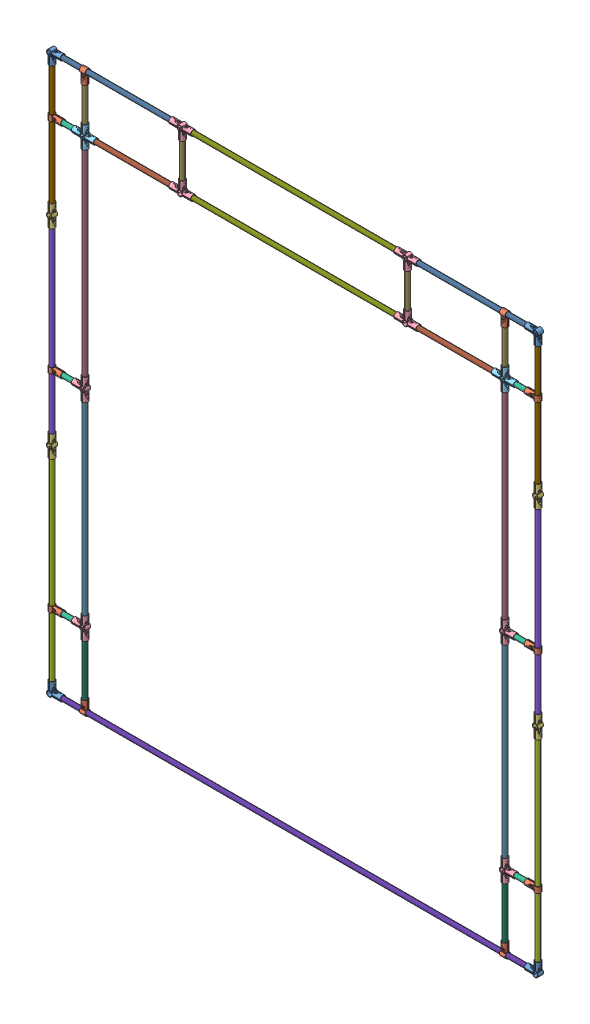
SolidWorks assembly End_Panel_Assembly, configuration Default. Lengths in mm.
Overall size (2924.59 3334.67 35.62).
57 component instances, 17 part files, 65 mates.
Components (placement in the parent):
- 28-25-3: 28-25 [2534T24] x (0 1 0) z (0 0 1) size (81.85 81.28 33.46)
- 28-20-9: 28-20 [2534T21] at (196 0 0) x (1 0 0) z (0 0 -1) size (33.53 82.55 34.1)
- 28-20-10: 28-20 [2534T21] at (0 436 0) x (0 -1 0) z (0 0 -1) size (33.53 82.55 34.1)
- 28-22-2: 28-22 [2534T25] at (0 1275 0) x (0 -1 0) z (0 0 1) size (130.05 34.67 33.46)
- 28-20-8: 28-20 [2534T21] at (0 1665 0) x (0 -1 0) z (0 0 -1) size (33.53 82.55 34.1)
- 24-25-4: 24-25 [2534T26] at (196 1665 0) x (0 1 0) z (0 0 -1) size (130.05 82.36 33.46)
- 28-22-3: 28-22 [2534T25] at (0 2461 0) x (0 -1 0) z (0 0 1) size (130.05 34.67 33.46)
- 28-24-3: 28-24 [2534T27] at (196 2965 0) size (130.05 130.05 33.46)
- 28-20-7: 28-20 [2534T21] at (0 2965 0) x (0 -1 0) z (0 0 -1) size (33.53 82.55 34.1)
- 24-25-24: 24-25 [2534T26] at (775 2965 0) x (1 0 0) z (0 0 -1) size (130.05 82.36 33.46)
- 28-25-5: 28-25 [2534T24] at (0 3300 0) size (81.85 81.28 33.46)
- 28-20-6: 28-20 [2534T21] at (196 3300 0) size (33.53 82.55 34.1)
- 24-25-25: 24-25 [2534T26] at (775 3300 0) size (130.05 82.36 33.46)
- 28-02-2: 28-02 [Default] at (43.381 436 0) size (110 25.4 25.4)
- 28-02-3: 28-02 [Default] at (43.381 1665 0) x (1 0 0) z (0 -0.125641 0.992076) size (110 25.4 25.4)
- 28-02-4: 28-02 [Default] at (43.381 2965 0) size (110 25.4 25.4)
- 28-03-1: 28-03 [Default] at (0 42.246 0) x (0 1 0) z (0 0 1) size (1190 25.4 25.4)
- 28-04-2: 28-04 [Default] at (0 2418 0) x (0 -1 0) z (-0.79674 0 -0.604323) size (1100 25.4 25.4)
- 28-05-1: 28-05 [Default] at (0 3255.754 0) x (0 -1 0) z (0.421273 0 0.906934) size (750 25.4 25.4)
- 28-06-1: 28-06 [Default] at (42.246 3300 0) size (690 25.4 25.4)
- 28-07-1: 28-07 [Default] at (240.5 2965 0) size (490 25.4 25.4)
- 28-08-1: 28-08 [Default] at (196 3254.619 0) x (0 -1 0) z (-0.507156 0 0.861854) size (245 25.4 25.4)
- 28-08-2: 28-08 [Default] at (775 3255 0) x (0 -1 0) z (0.98977 0 -0.14267) size (245 25.4 25.4)
- 28-09-1: 28-09 [Default] at (196 2920 0) x (0 -1 0) z (-0.937477 0 0.348048) size (1210 25.4 25.4)
- 28-10-1: 28-10 [Default] at (196 1620.5 0) x (0 -1 0) z (0.792816 0 0.609461) size (1140 25.4 25.4)
- 28-12-1: 28-12 [Default] at (196 45.881 0) x (0 1 0) z (0.833818 0 0.552039) size (345 25.4 25.4)
- 28-16-1: 28-16 [Default] at (819.25 3300 0) size (1250 25.4 25.4)
- 28-16-2: 28-16 [Default] at (819.5 2965 0) size (1250 25.4 25.4)
- 28-12-9: 28-12 [Default] at (2693 45.881 0) x (0 1 0) z (0.833818 0 -0.552039) size (345 25.4 25.4)
- 28-03-6: 28-03 [Default] at (2889 42.246 0) x (0 1 0) z (0 0 -1) size (1190 25.4 25.4)
- 28-25-15: 28-25 [2534T24] at (2889 0 0) x (0 1 0) z (0 0 -1) size (81.85 81.28 33.46)
- 28-20-27: 28-20 [2534T21] at (2693 0 0) x (1 0 0) z (0 0 -1) size (33.53 82.55 34.1)
- 28-02-17: 28-02 [Default] at (2845.619 436 0) x (-1 0 0) z (0 0 -1) size (110 25.4 25.4)
- 28-20-28: 28-20 [2534T21] at (2889 436 0) x (0 1 0) z (0 0 -1) size (33.53 82.55 34.1)
- 28-10-6: 28-10 [Default] at (2693 1620.5 0) x (0 -1 0) z (0.792816 0 -0.609461) size (1140 25.4 25.4)
- 28-22-12: 28-22 [2534T25] at (2889 1275 0) x (0 -1 0) z (0 0 -1) size (130.05 34.67 33.46)
- 28-04-7: 28-04 [Default] at (2889 2418 0) x (0 -1 0) z (-0.79674 0 0.604323) size (1100 25.4 25.4)
- 24-25-26: 24-25 [2534T26] at (2693 1665 0) x (0 1 0) z (0 0 1) size (130.05 82.36 33.46)
- 28-02-18: 28-02 [Default] at (2845.619 1665 0) x (-1 0 0) z (0 0.125641 -0.992076) size (110 25.4 25.4)
- 28-20-29: 28-20 [2534T21] at (2889 1665 0) x (0 1 0) z (0 0 -1) size (33.53 82.55 34.1)
- 28-09-6: 28-09 [Default] at (2693 2920 0) x (0 -1 0) z (-0.937477 0 -0.348048) size (1210 25.4 25.4)
- 28-22-13: 28-22 [2534T25] at (2889 2461 0) x (0 -1 0) z (0 0 -1) size (130.05 34.67 33.46)
- 28-05-6: 28-05 [Default] at (2889 3255.754 0) x (0 -1 0) z (0.421273 0 -0.906934) size (750 25.4 25.4)
- 28-08-11: 28-08 [Default] at (2114 3255 0) x (0 -1 0) z (0.98977 0 0.14267) size (245 25.4 25.4)
- 24-25-27: 24-25 [2534T26] at (2114 2965 0) x (-1 0 0) z (0 0 1) size (130.05 82.36 33.46)
- 28-07-6: 28-07 [Default] at (2648.5 2965 0) x (-1 0 0) z (0 0 -1) size (490 25.4 25.4)
- 28-24-13: 28-24 [2534T27] at (2693 2965 0) x (-1 0 0) z (0 0 -1) size (130.05 130.05 33.46)
- 28-02-19: 28-02 [Default] at (2845.619 2965 0) x (-1 0 0) z (0 0 -1) size (110 25.4 25.4)
- 28-20-30: 28-20 [2534T21] at (2889 2965 0) x (0 1 0) z (0 0 -1) size (33.53 82.55 34.1)
- 28-08-12: 28-08 [Default] at (2693 3254.619 0) x (0 -1 0) z (-0.507156 0 -0.861854) size (245 25.4 25.4)
- 28-25-16: 28-25 [2534T24] at (2889 3300 0) x (-1 0 0) z (0 0 -1) size (81.85 81.28 33.46)
- 28-20-31: 28-20 [2534T21] at (2693 3300 0) size (33.53 82.55 34.1)
- 28-06-6: 28-06 [Default] at (2846.754 3300 0) x (-1 0 0) z (0 0 -1) size (690 25.4 25.4)
- 24-25-28: 24-25 [2534T26] at (2114 3300 0) x (-1 0 0) z (0 0 -1) size (130.05 82.36 33.46)
- 28-17-1: 28-17 [Default] at (44.5 0 0) size (2800 25.4 25.4)
- 24-25-23: 24-25 [2534T26] at (196 436 0) x (0 1 0) z (0 0 -1) size (130.05 82.36 33.46)
- 24-25-29: 24-25 [2534T26] at (2693 436 0) x (0 1 0) z (0 0 1) size (130.05 82.36 33.46)
Mates (geometry in assembly coordinates):
- Coincident26: coincident: unknown of 3way connector-3
- Parallel15: parallel aligned: plane of 3way connector-3 through (0 64.516 0) normal (0 1 0)
- Parallel16: parallel aligned: plane of 3way connector-3 through (64.516 0 0) normal (1 0 0)
- Concentric12: concentric aligned: cylinder of 3way connector-3 through (64.516 0 0) axis (-1 0 0) radius 13.97; cylinder of Tee connector-2 through (212.764 0 0) axis (-1 0 0) radius 13.97
- Distance10: distance = 196 mm: unknown of Tee connector-2
- Parallel17: parallel aligned: plane of Tee connector-2 through (196 65.786 0) normal (0 1 0)
- Concentric18: concentric aligned: cylinder of 3way connector-3 through (0 64.516 0) axis (0 -1 0) radius 13.97; cylinder of Tee connector-3 through (0 452.764 0) axis (0 -1 0) radius 13.97
- Concentric19: concentric anti-aligned: cylinder of Tee connector-3 through (0 452.764 0) axis (0 -1 0) radius 13.97; cylinder of Cross-2 through (0 1209.976 0) axis (0 1 0) radius 13.97
- Distance13: distance = 1275 mm: unknown of Cross-2
- Concentric24: concentric anti-aligned: cylinder of Cross-2 through (0 1340.024 0) axis (0 -1 0) radius 13.97; cylinder of Tee connector-4 through (0 1648.236 0) axis (0 1 0) radius 13.97
- Concentric26: concentric anti-aligned: cylinder of Tee connector-4 through (65.786 1665 0) axis (-1 0 0) radius 13.97; cylinder of 5way connector-4 through (130.976 1665 0) axis (1 0 0) radius 13.97
- Concentric28: concentric anti-aligned: cylinder of Tee connector-4 through (0 1681.764 0) axis (0 -1 0) radius 13.97; cylinder of Cross-3 through (0 2395.976 0) axis (0 1 0) radius 13.97
- Parallel21: parallel aligned: plane of Tee connector-4 through (25.146 1665 12.065) normal (0 0 1); plane of Cross-3 through (0 2461 16.73) normal (0 0 1)
- Distance18: distance = 1186 mm: point of Cross-3; point of Cross-2
- Parallel22: parallel aligned: plane of Cross-3 through (0 2461 16.73) normal (0 0 1); plane of 6way connector-3 through (196 2965 16.73) normal (0 0 1)
- Concentric29: concentric anti-aligned: cylinder of 5way connector-4 through (196 1730.024 0) axis (0 -1 0) radius 13.97; cylinder of 6way connector-3 through (196 2899.976 0) axis (0 1 0) radius 13.97
- Distance19: distance = 1300 mm: point of 6way connector-3; point of 5way connector-4
- Concentric30: concentric aligned: cylinder of Cross-3 through (0 2526.024 0) axis (0 -1 0) radius 13.97; cylinder of Tee connector-5 through (0 2981.764 0) axis (0 -1 0) radius 13.97
- Concentric31: concentric anti-aligned: cylinder of 6way connector-3 through (130.976 2965 0) axis (1 0 0) radius 13.97; cylinder of Tee connector-5 through (65.786 2965 0) axis (-1 0 0) radius 13.97
- Concentric35: concentric anti-aligned: cylinder of 6way connector-3 through (261.024 2965 0) axis (-1 0 0) radius 13.97; cylinder of 5way connector-5 through (709.976 2965 0) axis (1 0 0) radius 13.97
- Concentric36: concentric aligned: cylinder of 3way connector-5 through (64.516 3300 0) axis (-1 0 0) radius 13.97; cylinder of Tee connector-6 through (212.764 3300 0) axis (-1 0 0) radius 13.97
- Concentric37: concentric anti-aligned: cylinder of Tee connector-5 through (0 2981.764 0) axis (0 -1 0) radius 13.97; cylinder of 3way connector-5 through (0 3235.484 0) axis (0 1 0) radius 13.97
- Concentric38: concentric anti-aligned: cylinder of 6way connector-3 through (196 3030.024 0) axis (0 -1 0) radius 13.97; cylinder of Tee connector-6 through (196 3234.214 0) axis (0 1 0) radius 13.97
- Distance22: distance = 335 mm: point of 3way connector-5; point of Tee connector-5
- Concentric39: concentric anti-aligned: cylinder of Tee connector-6 through (212.764 3300 0) axis (-1 0 0) radius 13.97; cylinder of 5way connector-6 through (709.976 3300 0) axis (1 0 0) radius 13.97
- Concentric41: concentric anti-aligned: cylinder of 5way connector-5 through (775 3030.024 0) axis (0 -1 0) radius 13.97; cylinder of 5way connector-6 through (775 3234.976 0) axis (0 1 0) radius 13.97
- Concentric44: concentric aligned: cylinder of Tee connector-4 through (65.786 1665 0) axis (-1 0 0) radius 13.97; cylinder of P2-3 through (153.381 1665 0) axis (-1 0 0) radius 12.7
- Width3: width anti-aligned: plane of P2-3 through (153.381 1665 0) normal (1 0 0); plane of P2-3 through (43.381 1665 0) normal (-1 0 0); plane of 5way connector-4 through (130.976 1665 0) normal (-1 0 0); plane of Tee connector-4 through (65.786 1665 0) normal (1 0 0)
- Width4: width anti-aligned: plane of P2-4 through (153.381 2965 0) normal (1 0 0); plane of P2-4 through (43.381 2965 0) normal (-1 0 0); plane of 6way connector-3 through (130.976 2965 0) normal (-1 0 0); plane of Tee connector-5 through (65.786 2965 0) normal (1 0 0)
- Concentric45: concentric aligned: cylinder of Tee connector-5 through (65.786 2965 0) axis (-1 0 0) radius 13.97; cylinder of P2-4 through (153.381 2965 0) axis (-1 0 0) radius 12.7
- Concentric46: concentric anti-aligned: cylinder of Cross-2 through (0 1209.976 0) axis (0 1 0) radius 13.97; cylinder of P3-1 through (0 1232.246 0) axis (0 -1 0) radius 12.7
- Width5: width aligned: plane of P3-1 through (0 42.246 0) normal (0 -1 0); plane of P3-1 through (0 1232.246 0) normal (0 1 0); plane of Cross-2 through (0 1209.976 0) normal (0 -1 0); plane of 3way connector-3 through (0 64.516 0) normal (0 1 0)
- Concentric47: concentric anti-aligned: cylinder of Cross-2 through (0 1340.024 0) axis (0 -1 0) radius 13.97; cylinder of P4-2 through (0 1318 0) axis (0 1 0) radius 12.7
- Width6: width anti-aligned: plane of P4-2 through (0 2418 0) normal (0 1 0); plane of P4-2 through (0 1318 0) normal (0 -1 0); plane of Cross-3 through (0 2395.976 0) normal (0 -1 0); plane of Cross-2 through (0 1340.024 0) normal (0 1 0)
- Concentric48: concentric anti-aligned: cylinder of Cross-3 through (0 2526.024 0) axis (0 -1 0) radius 13.97; cylinder of P5-1 through (0 2505.754 0) axis (0 1 0) radius 12.7
- Width7: width anti-aligned: plane of P5-1 through (0 3255.754 0) normal (0 1 0); plane of P5-1 through (0 2505.754 0) normal (0 -1 0); plane of 3way connector-5 through (0 3235.484 0) normal (0 -1 0); plane of Cross-3 through (0 2526.024 0) normal (0 1 0)
- Width8: width anti-aligned: plane of P6-1 through (42.246 3300 0) normal (-1 0 0); plane of P6-1 through (732.246 3300 0) normal (1 0 0); plane of 3way connector-5 through (64.516 3300 0) normal (1 0 0); plane of 5way connector-6 through (709.976 3300 0) normal (-1 0 0)
- Concentric49: concentric anti-aligned: cylinder of 5way connector-6 through (709.976 3300 0) axis (1 0 0) radius 13.97; cylinder of P6-1 through (732.246 3300 0) axis (-1 0 0) radius 12.7
- Width9: width anti-aligned: plane of P7-1 through (240.5 2965 0) normal (-1 0 0); plane of P7-1 through (730.5 2965 0) normal (1 0 0); plane of 6way connector-3 through (261.024 2965 0) normal (1 0 0); plane of 5way connector-5 through (709.976 2965 0) normal (-1 0 0)
- Concentric50: concentric anti-aligned: cylinder of 5way connector-5 through (709.976 2965 0) axis (1 0 0) radius 13.97; cylinder of P7-1 through (730.5 2965 0) axis (-1 0 0) radius 12.7
- Concentric51: concentric anti-aligned: cylinder of 6way connector-3 through (196 3030.024 0) axis (0 -1 0) radius 13.97; cylinder of P8-1 through (196 3009.619 0) axis (0 1 0) radius 12.7
- Concentric52: concentric anti-aligned: cylinder of 5way connector-5 through (775 3030.024 0) axis (0 -1 0) radius 13.97; cylinder of P8-2 through (775 3010 0) axis (0 1 0) radius 12.7
- Width10: width aligned: plane of P8-1 through (196 3254.619 0) normal (0 1 0); plane of P8-1 through (196 3009.619 0) normal (0 -1 0); plane of 6way connector-3 through (196 3030.024 0) normal (0 1 0); plane of Tee connector-6 through (196 3234.214 0) normal (0 -1 0)
- Width11: width anti-aligned: plane of P8-2 through (775 3255 0) normal (0 1 0); plane of P8-2 through (775 3010 0) normal (0 -1 0); plane of 5way connector-6 through (775 3234.976 0) normal (0 -1 0); plane of 5way connector-5 through (775 3030.024 0) normal (0 1 0)
- Concentric53: concentric anti-aligned: cylinder of 5way connector-4 through (196 1730.024 0) axis (0 -1 0) radius 13.97; cylinder of P9-1 through (196 1710 0) axis (0 1 0) radius 12.7
- Width12: width anti-aligned: plane of P9-1 through (196 1710 0) normal (0 -1 0); plane of P9-1 through (196 2920 0) normal (0 1 0); plane of 5way connector-4 through (196 1730.024 0) normal (0 1 0); plane of 6way connector-3 through (196 2899.976 0) normal (0 -1 0)
- Width20: width anti-aligned: plane of P16-1 through (2069.25 3300 0) normal (1 0 0); plane of P16-1 through (819.25 3300 0) normal (-1 0 0); plane of 5way connector-10 through (2048.976 3250 0) normal (-1 0 0); plane of 5way connector-6 through (840.024 3300 0) normal (1 0 0)
- Width21: width anti-aligned: plane of P16-2 through (2069.5 2965 0) normal (1 0 0); plane of P16-2 through (819.5 2965 0) normal (-1 0 0); plane of 5way connector-9 through (2048.976 2915 0) normal (-1 0 0); plane of 5way connector-5 through (840.024 2965 0) normal (1 0 0)
- Concentric62: concentric aligned: cylinder of 5way connector-6 through (840.024 3300 0) axis (-1 0 0) radius 13.97; cylinder of P16-1 through (2069.25 3300 0) axis (-1 0 0) radius 12.7
- Width22: width anti-aligned: plane of P17-1 through (44.5 0 0) normal (-1 0 0); plane of P17-1 through (2844.5 0 0) normal (1 0 0); plane of 3way connector-3 through (64.516 0 0) normal (1 0 0); plane of 3way connector-15 through (2824.484 0 0) normal (-1 0 0)
- Concentric63: concentric anti-aligned: cylinder of 3way connector-15 through (2824.484 0 0) axis (1 0 0) radius 13.97; cylinder of P17-1 through (2844.5 0 0) axis (-1 0 0) radius 12.7
- Distance23: distance = 196 mm: point of 5way connector-23; point of Tee connector-3
- Distance24: distance = 436 mm: point of 5way connector-23; point of Tee connector-2
- Coincident31: coincident: unknown of 5way connector-23
- Parallel26: parallel anti-aligned: plane of 5way connector-23 through (196 436 -16.73) normal (0 0 -1)
- Width23: width anti-aligned: plane of P2-2 through (43.381 436 0) normal (-1 0 0); plane of P2-2 through (153.381 436 0) normal (1 0 0); plane of Tee connector-3 through (65.786 436 0) normal (1 0 0); plane of 5way connector-23 through (130.976 436 0) normal (-1 0 0)
- Concentric66: concentric anti-aligned: cylinder of P2-2 through (153.381 436 0) axis (-1 0 0) radius 12.7; cylinder of 5way connector-23 through (130.976 436 0) axis (1 0 0) radius 13.97
- Width24: width anti-aligned: plane of P10-1 through (196 480.5 0) normal (0 -1 0); plane of P10-1 through (196 1620.5 0) normal (0 1 0); plane of 5way connector-23 through (196 501.024 0) normal (0 1 0); plane of 5way connector-4 through (196 1599.976 0) normal (0 -1 0)
- Concentric67: concentric aligned: cylinder of 5way connector-4 through (196 1599.976 0) axis (0 1 0) radius 13.97; cylinder of P10-1 through (196 480.5 0) axis (0 1 0) radius 12.7
- Width25: width anti-aligned: plane of P12-1 through (196 45.881 0) normal (0 -1 0); plane of P12-1 through (196 390.881 0) normal (0 1 0); plane of Tee connector-2 through (196 65.786 0) normal (0 1 0); plane of 5way connector-23 through (196 370.976 0) normal (0 -1 0)
- Concentric68: concentric anti-aligned: cylinder of P12-1 through (196 390.881 0) axis (0 -1 0) radius 12.7; cylinder of 5way connector-23 through (196 370.976 0) axis (0 1 0) radius 13.97
- Concentric69: concentric aligned: cylinder of Tee connector-2 through (196 65.786 0) axis (0 -1 0) radius 16.764; cylinder of P12-1 through (196 390.881 0) axis (0 -1 0) radius 12.7
- Distance25: distance = 1229 mm: point of 5way connector-4; point of 5way connector-23
- Concentric70: concentric anti-aligned: cylinder of P10-1 through (196 480.5 0) axis (0 1 0) radius 12.7; cylinder of 5way connector-23 through (196 501.024 0) axis (0 -1 0) radius 13.97
- Concentric71: concentric aligned: cylinder of 5way connector-5 through (840.024 2965 0) axis (-1 0 0) radius 13.97; cylinder of P16-2 through (2069.5 2965 0) axis (-1 0 0) radius 12.7
